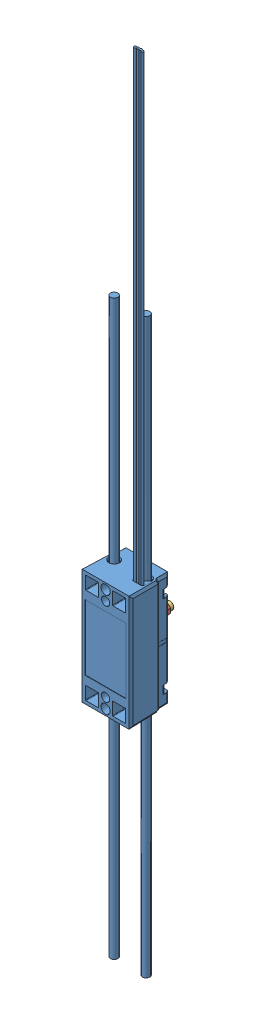
SolidWorks assembly Talon SRX (217-8080), configuration Default. Lengths in mm.
Overall size (30.47 491.79 30.05).
5 component instances, 3 part files, 0 mates.
Components (placement in the parent):
- Talon SRX (217-8080).step-1: Talon SRX (217-8080).step [Default] at origin size (30.47 491.79 30.05)
  - 217-8080-baseRev4.step-1: 217-8080-baseRev4.step [Default] at origin size (30.47 491.79 25.2)
  - 217-8080-002 Rev1.step-1: 217-8080-002 Rev1.step [Default] at (0 13.05 -9.65) x (1 0 0) z (0 -1 0) size (25.15 2.9 7.5)
  - 217-8080-005 Rev1_91251A105.step-1: 217-8080-005 Rev1_91251A105.step [Default] at (-9.525 13.05 -5.8875) size (4.65 4.65 7.61)
  - 217-8080-005 Rev1_91251A105.step-2: 217-8080-005 Rev1_91251A105.step [Default] at (9.525 13.05 -5.8875) size (4.65 4.65 7.61)
